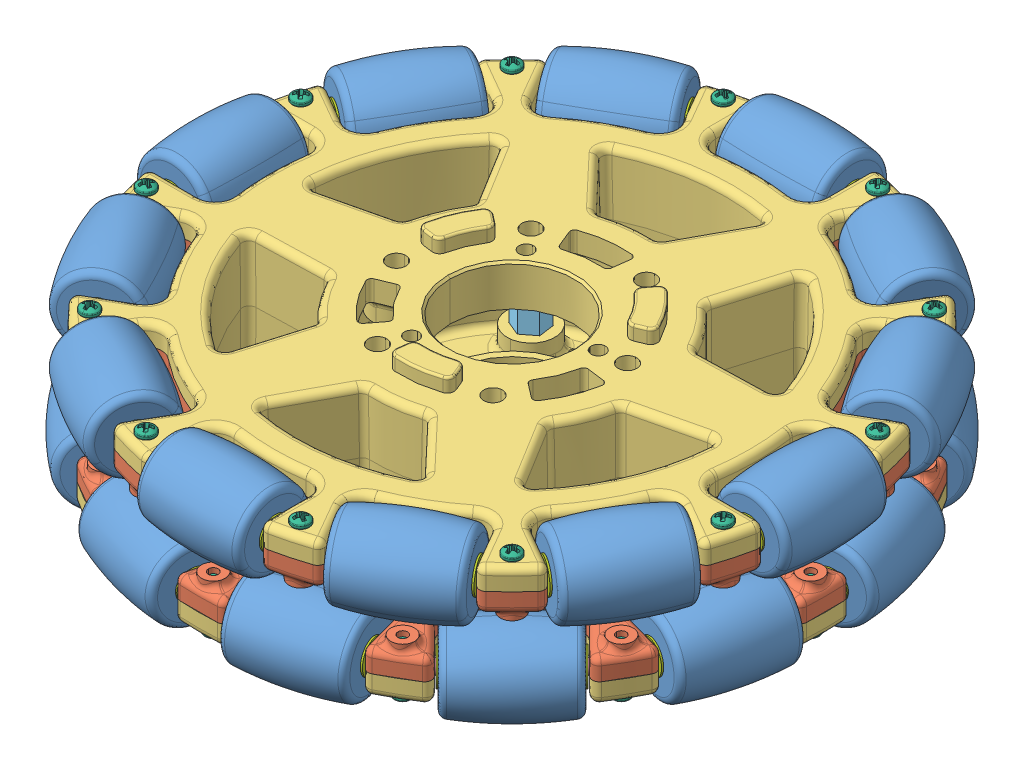
SolidWorks assembly 6 Omni-Directional Wheel (217-2585), configuration Default. Lengths in mm.
Overall size (174.23 42.44 174.23).
130 component instances, 7 part files, 0 mates.
Components (placement in the parent):
- 6 Omni-Directional Wheel (217-2585).step-1: 6 Omni-Directional Wheel (217-2585).step [Default] at origin size (174.23 42.44 174.23)
  - 217-2585-001 Rev1.step-1: 217-2585-001 Rev1.step [Default] at (0 9.4629 -66.8297) x (1 0 0) z (0 -0.857126 0.515108) size (24.13 18.81 18.81)
  - 217-2585-002 Rev1.step-1: 217-2585-002 Rev1.step [Default] x (1 0 0) z (0 1 0) size (145.16 145.16 19.05)
  - 217-2585-001 Rev1.step-2: 217-2585-001 Rev1.step [Default] at (47.2557 -9.4629 47.2557) x (-0.707107 0 0.707107) z (-0.700403 -0.137373 -0.700403) size (24.13 18.81 18.81)
  - 217-2585-001 Rev1.step-3: 217-2585-001 Rev1.step [Default] at (17.2968 -9.4629 64.5525) x (-0.965926 0 0.258819) z (-0.256365 -0.137373 -0.956768) size (24.13 18.81 18.81)
  - 217-2585-001 Rev1.step-4: 217-2585-001 Rev1.step [Default] at (-17.2968 -9.4629 64.5525) x (-0.965926 0 -0.258819) z (0.256365 -0.137373 -0.956768) size (24.13 18.81 18.81)
  - 217-2585-001 Rev1.step-5: 217-2585-001 Rev1.step [Default] at (-47.2557 -9.4629 47.2557) x (-0.707107 0 -0.707107) z (0.700403 -0.137373 -0.700403) size (24.13 18.81 18.81)
  - 217-2585-001 Rev1.step-6: 217-2585-001 Rev1.step [Default] at (-64.5525 -9.4629 17.2968) x (-0.258819 0 -0.965926) z (0.956768 -0.137373 -0.256365) size (24.13 18.81 18.81)
  - 217-2585-001 Rev1.step-7: 217-2585-001 Rev1.step [Default] at (-64.5525 -9.4629 -17.2968) x (0.258819 0 -0.965926) z (0.956768 -0.137373 0.256365) size (24.13 18.81 18.81)
  - 217-2585-001 Rev1.step-8: 217-2585-001 Rev1.step [Default] at (-47.2557 -9.4629 -47.2557) x (0.707107 0 -0.707107) z (0.700403 -0.137373 0.700403) size (24.13 18.81 18.81)
  - 217-2585-001 Rev1.step-9: 217-2585-001 Rev1.step [Default] at (-17.2968 -9.4629 -64.5525) x (0.965926 0 -0.258819) z (0.256365 -0.137373 0.956768) size (24.13 18.81 18.81)
  - 217-2585-001 Rev1.step-10: 217-2585-001 Rev1.step [Default] at (17.2968 -9.4629 -64.5525) x (0.965926 0 0.258819) z (-0.256365 -0.137373 0.956768) size (24.13 18.81 18.81)
  - 217-2585-001 Rev1.step-11: 217-2585-001 Rev1.step [Default] at (47.2557 -9.4629 -47.2557) x (0.707107 0 0.707107) z (-0.700403 -0.137373 0.700403) size (24.13 18.81 18.81)
  - 217-2585-001 Rev1.step-12: 217-2585-001 Rev1.step [Default] at (64.5525 -9.4629 -17.2968) x (0.258819 0 0.965926) z (-0.956768 -0.137373 0.256365) size (24.13 18.81 18.81)
  - 217-2585-001 Rev1.step-13: 217-2585-001 Rev1.step [Default] at (64.5525 -9.4629 17.2968) x (-0.258819 0 0.965926) z (-0.956768 -0.137373 -0.256365) size (24.13 18.81 18.81)
  - 217-2585-003 Rev2.step-1: 217-2585-003 Rev2.step [Default] at (0 -9.525 0) x (0.965926 0 -0.258819) z (0 -1 0) size (142.26 142.26 17.6)
  - 217-2585-004 Rev1.step-1: 217-2585-004 Rev1.step [Default] at (-57.9397 9.4629 -33.3049) x (0.5 0 -0.866025) z (-0.558431 0.764334 -0.32241) size (30.16 3 3)
  - 217-2585-004 Rev1.step-2: 217-2585-004 Rev1.step [Default] at (-64.5197 -9.4629 -17.4195) x (0.258819 0 -0.965926) z (-0.83871 -0.496046 -0.224732) size (30.16 3 3)
  - 217-2585-003 Rev2.step-2: 217-2585-003 Rev2.step [Default] at (0 9.525 0) x (-1 0 0) z (0 1 0) size (142.26 142.26 17.6)
  - 217-2585-004 Rev1.step-3: 217-2585-004 Rev1.step [Default] at (-33.5248 9.4629 -57.8127) x (0.866025 0 -0.5) z (-0.32241 0.764334 -0.558431) size (30.16 3 3)
  - 217-2585-004 Rev1.step-4: 217-2585-004 Rev1.step [Default] at (-0.127 9.4629 -66.8297) x (1 0 0) z (0 0.764334 -0.644821) size (30.16 3 3)
  - 217-2585-004 Rev1.step-5: 217-2585-004 Rev1.step [Default] at (33.3049 9.4629 -57.9397) x (0.866025 0 0.5) z (0.32241 0.764334 -0.558431) size (30.16 3 3)
  - 217-2585-004 Rev1.step-6: 217-2585-004 Rev1.step [Default] at (57.8127 9.4629 -33.5248) x (0.5 0 0.866025) z (0.558431 0.764334 -0.32241) size (30.16 3 3)
  - 217-2585-004 Rev1.step-7: 217-2585-004 Rev1.step [Default] at (66.8297 9.4629 -0.127) x (0 0 1) z (0.644821 0.764334 0) size (30.16 3 3)
  - 217-2585-004 Rev1.step-8: 217-2585-004 Rev1.step [Default] at (57.9397 9.4629 33.3049) x (-0.5 0 0.866025) z (0.558431 0.764334 0.32241) size (30.16 3 3)
  - 217-2585-004 Rev1.step-9: 217-2585-004 Rev1.step [Default] at (33.5248 9.4629 57.8127) x (-0.866025 0 0.5) z (0.32241 0.764334 0.558431) size (30.16 3 3)
  - 217-2585-004 Rev1.step-10: 217-2585-004 Rev1.step [Default] at (0.127 9.4629 66.8297) x (-1 0 0) z (0 0.764334 0.644821) size (30.16 3 3)
  - 217-2585-004 Rev1.step-11: 217-2585-004 Rev1.step [Default] at (-33.3049 9.4629 57.9397) x (-0.866025 0 -0.5) z (-0.32241 0.764334 0.558431) size (30.16 3 3)
  - 217-2585-004 Rev1.step-12: 217-2585-004 Rev1.step [Default] at (-57.8127 9.4629 33.5248) x (-0.5 0 -0.866025) z (-0.558431 0.764334 0.32241) size (30.16 3 3)
  - 217-2585-004 Rev1.step-13: 217-2585-004 Rev1.step [Default] at (-66.8297 9.4629 0.127) x (0 0 -1) z (-0.644821 0.764334 0) size (30.16 3 3)
  - 217-2585-004 Rev1.step-14: 217-2585-004 Rev1.step [Default] at (-47.1659 -9.4629 -47.3455) x (0.707107 0 -0.707107) z (-0.613978 -0.496046 -0.613978) size (30.16 3 3)
  - 217-2585-004 Rev1.step-15: 217-2585-004 Rev1.step [Default] at (-17.1741 -9.4629 -64.5854) x (0.965926 0 -0.258819) z (-0.224732 -0.496046 -0.83871) size (30.16 3 3)
  - 217-2585-004 Rev1.step-16: 217-2585-004 Rev1.step [Default] at (17.4195 -9.4629 -64.5197) x (0.965926 0 0.258819) z (0.224732 -0.496046 -0.83871) size (30.16 3 3)
  - 217-2585-004 Rev1.step-17: 217-2585-004 Rev1.step [Default] at (47.3455 -9.4629 -47.1659) x (0.707107 0 0.707107) z (0.613978 -0.496046 -0.613978) size (30.16 3 3)
  - 217-2585-004 Rev1.step-18: 217-2585-004 Rev1.step [Default] at (64.5854 -9.4629 -17.1741) x (0.258819 0 0.965926) z (0.83871 -0.496046 -0.224732) size (30.16 3 3)
  - 217-2585-004 Rev1.step-19: 217-2585-004 Rev1.step [Default] at (64.5197 -9.4629 17.4195) x (-0.258819 0 0.965926) z (0.83871 -0.496046 0.224732) size (30.16 3 3)
  - 217-2585-004 Rev1.step-20: 217-2585-004 Rev1.step [Default] at (47.1659 -9.4629 47.3455) x (-0.707107 0 0.707107) z (0.613978 -0.496046 0.613978) size (30.16 3 3)
  - 217-2585-004 Rev1.step-21: 217-2585-004 Rev1.step [Default] at (17.1741 -9.4629 64.5854) x (-0.965926 0 0.258819) z (0.224732 -0.496046 0.83871) size (30.16 3 3)
  - 217-2585-004 Rev1.step-22: 217-2585-004 Rev1.step [Default] at (-17.4195 -9.4629 64.5197) x (-0.965926 0 -0.258819) z (-0.224732 -0.496046 0.83871) size (30.16 3 3)
  - 217-2585-004 Rev1.step-23: 217-2585-004 Rev1.step [Default] at (-47.3455 -9.4629 47.1659) x (-0.707107 0 -0.707107) z (-0.613978 -0.496046 0.613978) size (30.16 3 3)
  - 217-2585-004 Rev1.step-24: 217-2585-004 Rev1.step [Default] at (-64.5854 -9.4629 17.1741) x (-0.258819 0 -0.965926) z (-0.83871 -0.496046 0.224732) size (30.16 3 3)
  - 217-2585-001 Rev1.step-14: 217-2585-001 Rev1.step [Default] at (33.4148 9.4629 -57.8762) x (0.866025 0 0.5) z (-0.257554 -0.857126 0.446096) size (24.13 18.81 18.81)
  - 217-2585-001 Rev1.step-15: 217-2585-001 Rev1.step [Default] at (57.8762 9.4629 -33.4148) x (0.5 0 0.866025) z (-0.446096 -0.857126 0.257554) size (24.13 18.81 18.81)
  - 217-2585-001 Rev1.step-16: 217-2585-001 Rev1.step [Default] at (66.8297 9.4629 0) x (0 0 1) z (-0.515108 -0.857126 0) size (24.13 18.81 18.81)
  - 217-2585-001 Rev1.step-17: 217-2585-001 Rev1.step [Default] at (57.8762 9.4629 33.4148) x (-0.5 0 0.866025) z (-0.446096 -0.857126 -0.257554) size (24.13 18.81 18.81)
  - 217-2585-001 Rev1.step-18: 217-2585-001 Rev1.step [Default] at (33.4148 9.4629 57.8762) x (-0.866025 0 0.5) z (-0.257554 -0.857126 -0.446096) size (24.13 18.81 18.81)
  - 217-2585-001 Rev1.step-19: 217-2585-001 Rev1.step [Default] at (0 9.4629 66.8297) x (-1 0 0) z (0 -0.857126 -0.515108) size (24.13 18.81 18.81)
  - 217-2585-001 Rev1.step-20: 217-2585-001 Rev1.step [Default] at (-33.4148 9.4629 57.8762) x (-0.866025 0 -0.5) z (0.257554 -0.857126 -0.446096) size (24.13 18.81 18.81)
  - 217-2585-001 Rev1.step-21: 217-2585-001 Rev1.step [Default] at (-57.8762 9.4629 33.4148) x (-0.5 0 -0.866025) z (0.446096 -0.857126 -0.257554) size (24.13 18.81 18.81)
  - 217-2585-001 Rev1.step-22: 217-2585-001 Rev1.step [Default] at (-66.8297 9.4629 0) x (0 0 -1) z (0.515108 -0.857126 0) size (24.13 18.81 18.81)
  - 217-2585-001 Rev1.step-23: 217-2585-001 Rev1.step [Default] at (-57.8762 9.4629 -33.4148) x (0.5 0 -0.866025) z (0.446096 -0.857126 0.257554) size (24.13 18.81 18.81)
  - 217-2585-001 Rev1.step-24: 217-2585-001 Rev1.step [Default] at (-33.4148 9.4629 -57.8762) x (0.866025 0 -0.5) z (0.257554 -0.857126 0.446096) size (24.13 18.81 18.81)
  - BEAM-0750.step-1: BEAM-0750.step [Default] at (-23.6088 0 3.1082) x (0.793353 0 -0.608761) z (0.608761 0 0.793353) size (7.34 19.05 7.34)
  - BEAM-0750.step-2: BEAM-0750.step [Default] at (-14.4961 0 -18.8917) x (0.92388 0 0.382683) z (-0.382683 0 0.92388) size (7.34 19.05 7.34)
  - BEAM-0750.step-3: BEAM-0750.step [Default] at (9.1126 0 -21.9999) x (0.130526 0 0.991445) z (-0.991445 0 0.130526) size (7.34 19.05 7.34)
  - BEAM-0750.step-4: BEAM-0750.step [Default] at (23.6088 0 -3.1082) x (-0.793353 0 0.608761) z (-0.608761 0 -0.793353) size (7.34 19.05 7.34)
  - BEAM-0750.step-5: BEAM-0750.step [Default] at (14.4961 0 18.8917) x (-0.92388 0 -0.382683) z (0.382683 0 -0.92388) size (7.34 19.05 7.34)
  - BEAM-0750.step-6: BEAM-0750.step [Default] at (-9.1126 0 21.9999) x (-0.130526 0 -0.991445) z (0.991445 0 -0.130526) size (7.34 19.05 7.34)
  - 90116A020_90116A020.step-1: 90116A020_90116A020.step [Default] at (34.544 -4.2875 -59.832) x (0.956072 0 -0.293131) z (0 -1 0) size (4 4 11.61)
  - 90116A020_90116A020.step-2: 90116A020_90116A020.step [Default] at (59.832 -4.2875 -34.544) x (0.974548 0 0.224177) z (0 -1 0) size (4 4 11.61)
  - 90116A020_90116A020.step-3: 90116A020_90116A020.step [Default] at (69.088 -4.2875 0) x (0.731895 0 0.681417) z (0 -1 0) size (4 4 11.61)
  - 90116A020_90116A020.step-4: 90116A020_90116A020.step [Default] at (59.832 -4.2875 34.544) x (0.293131 0 0.956072) z (0 -1 0) size (4 4 11.61)
  - 90116A020_90116A020.step-5: 90116A020_90116A020.step [Default] at (34.544 -4.2875 59.832) x (-0.224177 0 0.974548) z (0 -1 0) size (4 4 11.61)
  - 90116A020_90116A020.step-6: 90116A020_90116A020.step [Default] at (0 -4.2875 69.088) x (-0.681417 0 0.731895) z (0 -1 0) size (4 4 11.61)
  - 90116A020_90116A020.step-7: 90116A020_90116A020.step [Default] at (-34.544 -4.2875 59.832) x (-0.956072 0 0.293131) z (0 -1 0) size (4 4 11.61)
  - 90116A020_90116A020.step-8: 90116A020_90116A020.step [Default] at (-59.832 -4.2875 34.544) x (-0.974548 0 -0.224177) z (0 -1 0) size (4 4 11.61)
  - 90116A020_90116A020.step-9: 90116A020_90116A020.step [Default] at (-69.088 -4.2875 0) x (-0.731895 0 -0.681417) z (0 -1 0) size (4 4 11.61)
  - 90116A020_90116A020.step-10: 90116A020_90116A020.step [Default] at (-59.832 -4.2875 -34.544) x (-0.293131 0 -0.956072) z (0 -1 0) size (4 4 11.61)
  - 90116A020_90116A020.step-11: 90116A020_90116A020.step [Default] at (-34.544 -4.2875 -59.832) x (0.224177 0 -0.974548) z (0 -1 0) size (4 4 11.61)
  - 90116A020_90116A020.step-12: 90116A020_90116A020.step [Default] at (0 -4.2875 -69.088) x (0.681417 0 -0.731895) z (0 -1 0) size (4 4 11.61)
  - 90116A020_90116A020.step-13: 90116A020_90116A020.step [Default] at (66.7339 4.2875 -17.8813) x (-0.938474 0 -0.34535) z (0 1 0) size (4 4 11.61)
  - 90116A020_90116A020.step-14: 90116A020_90116A020.step [Default] at (66.7339 4.2875 17.8813) x (-0.640068 0 -0.768319) z (0 1 0) size (4 4 11.61)
  - 90116A020_90116A020.step-15: 90116A020_90116A020.step [Default] at (48.8526 4.2875 48.8526) x (-0.170155 0 -0.985417) z (0 1 0) size (4 4 11.61)
  - 90116A020_90116A020.step-16: 90116A020_90116A020.step [Default] at (17.8813 4.2875 66.7339) x (0.34535 0 -0.938474) z (0 1 0) size (4 4 11.61)
  - 90116A020_90116A020.step-17: 90116A020_90116A020.step [Default] at (-17.8813 4.2875 66.7339) x (0.768319 0 -0.640068) z (0 1 0) size (4 4 11.61)
  - 90116A020_90116A020.step-18: 90116A020_90116A020.step [Default] at (-48.8526 4.2875 48.8526) x (0.985417 0 -0.170155) z (0 1 0) size (4 4 11.61)
  - 90116A020_90116A020.step-19: 90116A020_90116A020.step [Default] at (-66.7339 4.2875 17.8813) x (0.938474 0 0.34535) z (0 1 0) size (4 4 11.61)
  - 90116A020_90116A020.step-20: 90116A020_90116A020.step [Default] at (-66.7339 4.2875 -17.8813) x (0.640068 0 0.768319) z (0 1 0) size (4 4 11.61)
  - 90116A020_90116A020.step-21: 90116A020_90116A020.step [Default] at (-48.8526 4.2875 -48.8526) x (0.170155 0 0.985417) z (0 1 0) size (4 4 11.61)
  - 90116A020_90116A020.step-22: 90116A020_90116A020.step [Default] at (-17.8813 4.2875 -66.7339) x (-0.34535 0 0.938474) z (0 1 0) size (4 4 11.61)
  - 90116A020_90116A020.step-23: 90116A020_90116A020.step [Default] at (17.8813 4.2875 -66.7339) x (-0.768319 0 0.640068) z (0 1 0) size (4 4 11.61)
  - 90116A020_90116A020.step-24: 90116A020_90116A020.step [Default] at (48.8526 4.2875 -48.8526) x (-0.985417 0 0.170155) z (0 1 0) size (4 4 11.61)
  - 217-2584-005 Rev1 A.step-1: 217-2584-005 Rev1 A.step [Default] at (-7.3025 9.4629 -66.8297) x (0 -0.523633 0.851944) z (-1 0 0) size (7.38 7.38 9.92)
  - 217-2584-005 Rev1 A.step-2: 217-2584-005 Rev1 A.step [Default] at (7.3025 9.4629 -66.8297) x (0 -0.987336 0.15864) z (1 0 0) size (7.38 7.38 9.92)
  - 217-2584-005 Rev1 A.step-3: 217-2584-005 Rev1 A.step [Default] at (-24.3505 -9.4629 -62.6625) x (-0.242217 -0.352388 -0.903966) z (-0.965926 0 0.258819) size (7.38 7.38 9.92)
  - 217-2584-005 Rev1 A.step-4: 217-2584-005 Rev1 A.step [Default] at (-10.2431 -9.4629 -66.4425) x (0.244105 0.332373 0.911011) z (0.965926 0 -0.258819) size (7.38 7.38 9.92)
  - 217-2584-005 Rev1 A.step-5: 217-2584-005 Rev1 A.step [Default] at (10.2431 -9.4629 -66.4425) x (0.242217 -0.352388 -0.903966) z (-0.965926 0 -0.258819) size (7.38 7.38 9.92)
  - 217-2584-005 Rev1 A.step-6: 217-2584-005 Rev1 A.step [Default] at (42.0921 -9.4629 -52.4194) x (0.661749 -0.352388 -0.661749) z (-0.707107 0 -0.707107) size (7.38 7.38 9.92)
  - 217-2584-005 Rev1 A.step-7: 217-2584-005 Rev1 A.step [Default] at (62.6625 -9.4629 -24.3505) x (0.903966 -0.352388 -0.242217) z (-0.258819 0 -0.965926) size (7.38 7.38 9.92)
  - 217-2584-005 Rev1 A.step-8: 217-2584-005 Rev1 A.step [Default] at (66.4425 -9.4629 10.2431) x (0.903966 -0.352388 0.242217) z (0.258819 0 -0.965926) size (7.38 7.38 9.92)
  - 217-2584-005 Rev1 A.step-9: 217-2584-005 Rev1 A.step [Default] at (52.4194 -9.4629 42.0921) x (0.661749 -0.352388 0.661749) z (0.707107 0 -0.707107) size (7.38 7.38 9.92)
  - 217-2584-005 Rev1 A.step-10: 217-2584-005 Rev1 A.step [Default] at (24.3505 -9.4629 62.6625) x (0.242217 -0.352388 0.903966) z (0.965926 0 -0.258819) size (7.38 7.38 9.92)
  - 217-2584-005 Rev1 A.step-11: 217-2584-005 Rev1 A.step [Default] at (-10.2431 -9.4629 66.4425) x (-0.242217 -0.352388 0.903966) z (0.965926 0 0.258819) size (7.38 7.38 9.92)
  - 217-2584-005 Rev1 A.step-12: 217-2584-005 Rev1 A.step [Default] at (-42.0921 -9.4629 52.4194) x (-0.661749 -0.352388 0.661749) z (0.707107 0 0.707107) size (7.38 7.38 9.92)
  - 217-2584-005 Rev1 A.step-13: 217-2584-005 Rev1 A.step [Default] at (-62.6625 -9.4629 24.3505) x (-0.903966 -0.352388 0.242217) z (0.258819 0 0.965926) size (7.38 7.38 9.92)
  - 217-2584-005 Rev1 A.step-14: 217-2584-005 Rev1 A.step [Default] at (-66.4425 -9.4629 -10.2431) x (-0.903966 -0.352388 -0.242217) z (-0.258819 0 0.965926) size (7.38 7.38 9.92)
  - 217-2584-005 Rev1 A.step-15: 217-2584-005 Rev1 A.step [Default] at (-52.4194 -9.4629 -42.0921) x (-0.661749 -0.352388 -0.661749) z (-0.707107 0 0.707107) size (7.38 7.38 9.92)
  - 217-2584-005 Rev1 A.step-16: 217-2584-005 Rev1 A.step [Default] at (24.3505 -9.4629 -62.6625) x (-0.244105 0.332373 0.911011) z (0.965926 0 0.258819) size (7.38 7.38 9.92)
  - 217-2584-005 Rev1 A.step-17: 217-2584-005 Rev1 A.step [Default] at (52.4194 -9.4629 -42.0921) x (-0.666906 0.332373 0.666906) z (0.707107 0 0.707107) size (7.38 7.38 9.92)
  - 217-2584-005 Rev1 A.step-18: 217-2584-005 Rev1 A.step [Default] at (66.4425 -9.4629 -10.2431) x (-0.911011 0.332373 0.244105) z (0.258819 0 0.965926) size (7.38 7.38 9.92)
  - 217-2584-005 Rev1 A.step-19: 217-2584-005 Rev1 A.step [Default] at (62.6625 -9.4629 24.3505) x (-0.911011 0.332373 -0.244105) z (-0.258819 0 0.965926) size (7.38 7.38 9.92)
  - 217-2584-005 Rev1 A.step-20: 217-2584-005 Rev1 A.step [Default] at (42.0921 -9.4629 52.4194) x (-0.666906 0.332373 -0.666906) z (-0.707107 0 0.707107) size (7.38 7.38 9.92)
  - 217-2584-005 Rev1 A.step-21: 217-2584-005 Rev1 A.step [Default] at (10.2431 -9.4629 66.4425) x (-0.244105 0.332373 -0.911011) z (-0.965926 0 0.258819) size (7.38 7.38 9.92)
  - 217-2584-005 Rev1 A.step-22: 217-2584-005 Rev1 A.step [Default] at (-24.3505 -9.4629 62.6625) x (0.244105 0.332373 -0.911011) z (-0.965926 0 -0.258819) size (7.38 7.38 9.92)
  - 217-2584-005 Rev1 A.step-23: 217-2584-005 Rev1 A.step [Default] at (-52.4194 -9.4629 42.0921) x (0.666906 0.332373 -0.666906) z (-0.707107 0 -0.707107) size (7.38 7.38 9.92)
  - 217-2584-005 Rev1 A.step-24: 217-2584-005 Rev1 A.step [Default] at (-66.4425 -9.4629 10.2431) x (0.911011 0.332373 -0.244105) z (-0.258819 0 -0.965926) size (7.38 7.38 9.92)
  - 217-2584-005 Rev1 A.step-25: 217-2584-005 Rev1 A.step [Default] at (-62.6625 -9.4629 -24.3505) x (0.911011 0.332373 0.244105) z (0.258819 0 -0.965926) size (7.38 7.38 9.92)
  - 217-2584-005 Rev1 A.step-26: 217-2584-005 Rev1 A.step [Default] at (-42.0921 -9.4629 -52.4194) x (0.666906 0.332373 0.666906) z (0.707107 0 -0.707107) size (7.38 7.38 9.92)
  - 217-2584-005 Rev1 A.step-27: 217-2584-005 Rev1 A.step [Default] at (39.739 9.4629 -54.225) x (-0.07932 -0.987336 0.137386) z (0.866025 0 0.5) size (7.38 7.38 9.92)
  - 217-2584-005 Rev1 A.step-28: 217-2584-005 Rev1 A.step [Default] at (61.5275 9.4629 -27.0907) x (-0.137386 -0.987336 0.07932) z (0.5 0 0.866025) size (7.38 7.38 9.92)
  - 217-2584-005 Rev1 A.step-29: 217-2584-005 Rev1 A.step [Default] at (66.8297 9.4629 7.3025) x (-0.15864 -0.987336 0) z (0 0 1) size (7.38 7.38 9.92)
  - 217-2584-005 Rev1 A.step-30: 217-2584-005 Rev1 A.step [Default] at (54.225 9.4629 39.739) x (-0.137386 -0.987336 -0.07932) z (-0.5 0 0.866025) size (7.38 7.38 9.92)
  - 217-2584-005 Rev1 A.step-31: 217-2584-005 Rev1 A.step [Default] at (27.0907 9.4629 61.5275) x (-0.07932 -0.987336 -0.137386) z (-0.866025 0 0.5) size (7.38 7.38 9.92)
  - 217-2584-005 Rev1 A.step-32: 217-2584-005 Rev1 A.step [Default] at (-7.3025 9.4629 66.8297) x (0 -0.987336 -0.15864) z (-1 0 0) size (7.38 7.38 9.92)
  - 217-2584-005 Rev1 A.step-33: 217-2584-005 Rev1 A.step [Default] at (-39.739 9.4629 54.225) x (0.07932 -0.987336 -0.137386) z (-0.866025 0 -0.5) size (7.38 7.38 9.92)
  - 217-2584-005 Rev1 A.step-34: 217-2584-005 Rev1 A.step [Default] at (-61.5275 9.4629 27.0907) x (0.137386 -0.987336 -0.07932) z (-0.5 0 -0.866025) size (7.38 7.38 9.92)
  - 217-2584-005 Rev1 A.step-35: 217-2584-005 Rev1 A.step [Default] at (-66.8297 9.4629 -7.3025) x (0.15864 -0.987336 0) z (0 0 -1) size (7.38 7.38 9.92)
  - 217-2584-005 Rev1 A.step-36: 217-2584-005 Rev1 A.step [Default] at (-54.225 9.4629 -39.739) x (0.137386 -0.987336 0.07932) z (0.5 0 -0.866025) size (7.38 7.38 9.92)
  - 217-2584-005 Rev1 A.step-37: 217-2584-005 Rev1 A.step [Default] at (-27.0907 9.4629 -61.5275) x (0.07932 -0.987336 0.137386) z (0.866025 0 -0.5) size (7.38 7.38 9.92)
  - 217-2584-005 Rev1 A.step-38: 217-2584-005 Rev1 A.step [Default] at (27.0907 9.4629 -61.5275) x (-0.425972 -0.523633 0.737805) z (-0.866025 0 -0.5) size (7.38 7.38 9.92)
  - 217-2584-005 Rev1 A.step-39: 217-2584-005 Rev1 A.step [Default] at (54.225 9.4629 -39.739) x (-0.737805 -0.523633 0.425972) z (-0.5 0 -0.866025) size (7.38 7.38 9.92)
  - 217-2584-005 Rev1 A.step-40: 217-2584-005 Rev1 A.step [Default] at (66.8297 9.4629 -7.3025) x (-0.851944 -0.523633 0) z (0 0 -1) size (7.38 7.38 9.92)
  - 217-2584-005 Rev1 A.step-41: 217-2584-005 Rev1 A.step [Default] at (61.5275 9.4629 27.0907) x (-0.737805 -0.523633 -0.425972) z (0.5 0 -0.866025) size (7.38 7.38 9.92)
  - 217-2584-005 Rev1 A.step-42: 217-2584-005 Rev1 A.step [Default] at (39.739 9.4629 54.225) x (-0.425972 -0.523633 -0.737805) z (0.866025 0 -0.5) size (7.38 7.38 9.92)
  - 217-2584-005 Rev1 A.step-43: 217-2584-005 Rev1 A.step [Default] at (7.3025 9.4629 66.8297) x (0 -0.523633 -0.851944) z (1 0 0) size (7.38 7.38 9.92)
  - 217-2584-005 Rev1 A.step-44: 217-2584-005 Rev1 A.step [Default] at (-27.0907 9.4629 61.5275) x (0.425972 -0.523633 -0.737805) z (0.866025 0 0.5) size (7.38 7.38 9.92)
  - 217-2584-005 Rev1 A.step-45: 217-2584-005 Rev1 A.step [Default] at (-54.225 9.4629 39.739) x (0.737805 -0.523633 -0.425972) z (0.5 0 0.866025) size (7.38 7.38 9.92)
  - 217-2584-005 Rev1 A.step-46: 217-2584-005 Rev1 A.step [Default] at (-66.8297 9.4629 7.3025) x (0.851944 -0.523633 0) z (0 0 1) size (7.38 7.38 9.92)
  - 217-2584-005 Rev1 A.step-47: 217-2584-005 Rev1 A.step [Default] at (-61.5275 9.4629 -27.0907) x (0.737805 -0.523633 0.425972) z (-0.5 0 0.866025) size (7.38 7.38 9.92)
  - 217-2584-005 Rev1 A.step-48: 217-2584-005 Rev1 A.step [Default] at (-39.739 9.4629 -54.225) x (0.425972 -0.523633 0.737805) z (-0.866025 0 0.5) size (7.38 7.38 9.92)
